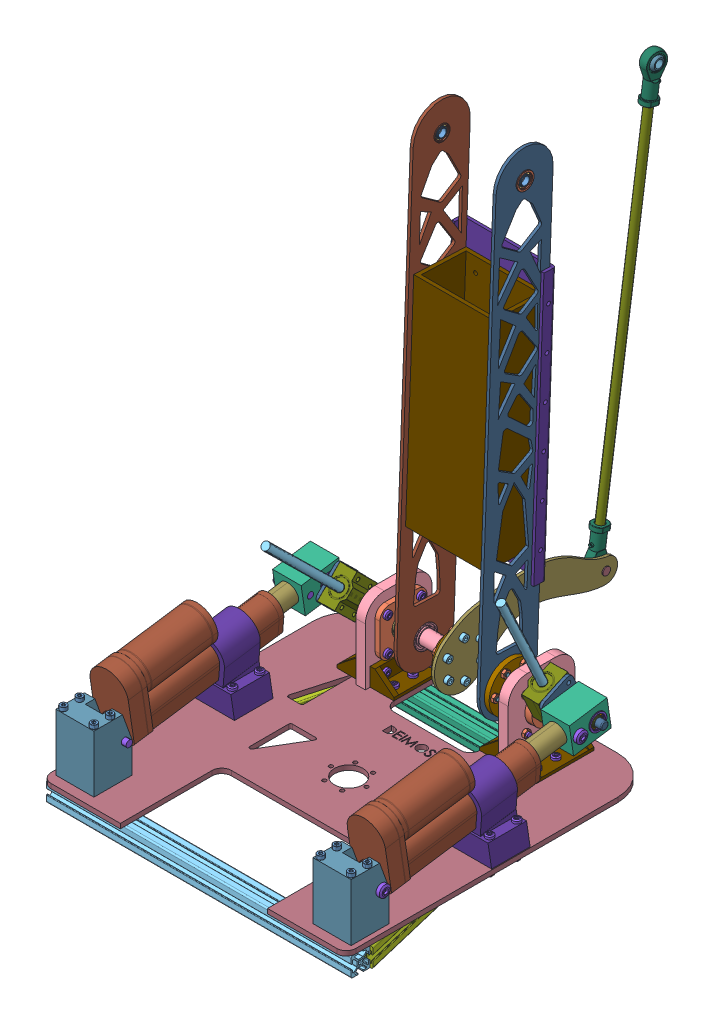
SolidWorks assembly Base + Link1 Final assembly, configuration Default. Lengths in mm. (continued)
Mates (geometry in assembly coordinates): (continued)
- Concentric128: concentric anti-aligned: cylinder of l bracket_arm base flang-4 through (213.5714 103.6403 167.5796) axis (1 0 0) radius 1.6729; cylinder of hexalobular socket pan head_iso-19 through (193.5714 103.6403 167.5796) axis (-1 0 0) radius 2.35
- Coincident132: coincident anti-aligned: plane of l bracket_arm base flang-4 through (218.5714 111.6403 178.5796) normal (1 0 0); plane of hexalobular socket pan head_iso-19 through (218.5714 101.2903 167.5796) normal (-1 0 0)
- Concentric129: concentric anti-aligned: cylinder of l bracket_arm base flang-4 through (213.5714 103.6403 148.5796) axis (1 0 0) radius 1.6729; cylinder of hexalobular socket pan head_iso-20 through (193.5714 103.6403 148.5796) axis (-1 0 0) radius 2.35
- Coincident133: coincident anti-aligned: plane of l bracket_arm base flang-4 through (218.5714 111.6403 178.5796) normal (1 0 0); plane of hexalobular socket pan head_iso-20 through (218.5714 101.2903 148.5796) normal (-1 0 0)
- Concentric130: concentric anti-aligned: cylinder of l bracket_arm base flang-4 through (213.5714 103.6403 129.5796) axis (1 0 0) radius 1.6729; cylinder of hexalobular socket pan head_iso-21 through (193.5714 103.6403 129.5796) axis (-1 0 0) radius 2.35
- Coincident134: coincident anti-aligned: plane of l bracket_arm base flang-4 through (218.5714 111.6403 178.5796) normal (1 0 0); plane of hexalobular socket pan head_iso-21 through (218.5714 101.2903 129.5796) normal (-1 0 0)
- Concentric131: concentric anti-aligned: cylinder of base bearing assambly-2/base shaft bearing housing-1 through (358.5714 155.1403 131.0796) axis (-1 0 0) radius 2; cylinder of hexalobular socket pan head_iso-23 through (368.5714 155.1403 131.0796) axis (1 0 0) radius 2.35
- Coincident135: coincident anti-aligned: plane of base bearing assambly-2/base shaft bearing housing-1 through (348.5714 149.6403 148.5796) normal (-1 0 0); plane of hexalobular socket pan head_iso-23 through (348.5714 157.4903 131.0796) normal (1 0 0)
- Concentric132: concentric anti-aligned: cylinder of base bearing assambly-2/base shaft bearing housing-1 through (358.5714 155.1403 166.0796) axis (-1 0 0) radius 2; cylinder of hexalobular socket pan head_iso-24 through (368.5714 155.1403 166.0796) axis (1 0 0) radius 2.35
- Coincident136: coincident anti-aligned: plane of base bearing assambly-2/base shaft bearing housing-1 through (348.5714 149.6403 148.5796) normal (-1 0 0); plane of hexalobular socket pan head_iso-24 through (348.5714 157.4903 166.0796) normal (1 0 0)
- Concentric133: concentric anti-aligned: cylinder of base bearing assambly-2/base shaft bearing housing-1 through (358.5714 120.1403 131.0796) axis (-1 0 0) radius 2; cylinder of hexalobular socket pan head_iso-25 through (368.5714 120.1403 131.0796) axis (1 0 0) radius 2.35
- Coincident137: coincident anti-aligned: plane of base bearing assambly-2/base shaft bearing housing-1 through (348.5714 149.6403 148.5796) normal (-1 0 0); plane of hexalobular socket pan head_iso-25 through (348.5714 122.4903 131.0796) normal (1 0 0)
- Concentric134: concentric anti-aligned: cylinder of base bearing assambly-2/base shaft bearing housing-1 through (358.5714 120.1403 166.0796) axis (-1 0 0) radius 2; cylinder of hexalobular socket pan head_iso-26 through (368.5714 120.1403 166.0796) axis (1 0 0) radius 2.35
- Coincident138: coincident anti-aligned: plane of base bearing assambly-2/base shaft bearing housing-1 through (348.5714 149.6403 148.5796) normal (-1 0 0); plane of hexalobular socket pan head_iso-26 through (348.5714 122.4903 166.0796) normal (1 0 0)
- Concentric1351: concentric anti-aligned: cylinder of base bearing assambly-1/base shaft bearing housing-1 through (208.5714 120.1403 131.0796) axis (1 0 0) radius 2; cylinder of hexalobular socket pan head_iso-27 through (198.5714 120.1403 131.0796) axis (-1 0 0) radius 2.35
- Coincident1391: coincident anti-aligned: plane of base bearing assambly-1/base shaft bearing housing-1 through (218.5714 149.6403 148.5796) normal (1 0 0); plane of hexalobular socket pan head_iso-27 through (218.5714 117.7903 131.0796) normal (-1 0 0)
- Concentric136: concentric anti-aligned: cylinder of base bearing assambly-1/base shaft bearing housing-1 through (208.5714 155.1403 131.0796) axis (1 0 0) radius 2; cylinder of hexalobular socket pan head_iso-28 through (198.5714 155.1403 131.0796) axis (-1 0 0) radius 2.35
- Coincident140: coincident anti-aligned: plane of base bearing assambly-1/base shaft bearing housing-1 through (218.5714 149.6403 148.5796) normal (1 0 0); plane of hexalobular socket pan head_iso-28 through (218.5714 152.7903 131.0796) normal (-1 0 0)
- Concentric137: concentric anti-aligned: cylinder of base bearing assambly-1/base shaft bearing housing-1 through (208.5714 155.1403 166.0796) axis (1 0 0) radius 2; cylinder of hexalobular socket pan head_iso-29 through (198.5714 155.1403 166.0796) axis (-1 0 0) radius 2.35
- Coincident141: coincident anti-aligned: plane of base bearing assambly-1/base shaft bearing housing-1 through (218.5714 149.6403 148.5796) normal (1 0 0); plane of hexalobular socket pan head_iso-29 through (218.5714 152.7903 166.0796) normal (-1 0 0)
- Concentric138: concentric anti-aligned: cylinder of base bearing assambly-1/base shaft bearing housing-1 through (208.5714 120.1403 166.0796) axis (1 0 0) radius 2; cylinder of hexalobular socket pan head_iso-30 through (198.5714 120.1403 166.0796) axis (-1 0 0) radius 2.35
- Coincident142: coincident anti-aligned: plane of base bearing assambly-1/base shaft bearing housing-1 through (218.5714 149.6403 148.5796) normal (1 0 0); plane of hexalobular socket pan head_iso-30 through (218.5714 117.7903 166.0796) normal (-1 0 0)
- Concentric139: concentric anti-aligned: cylinder of linear_acutator_holder-1 through (437.6971 82.0703 277.3153) axis (0 1 0) radius 2; cylinder of hexalobular socket pan head_iso-32 through (437.6971 83.0703 277.3153) axis (0 -1 0) radius 2.35
- Coincident143: coincident anti-aligned: plane of linear_acutator_holder-1 through (394.6971 118.0703 243.4855) normal (0 1 0); plane of hexalobular socket pan head_iso-32 through (440.0471 118.0703 277.3153) normal (0 -1 0)
- Concentric140: concentric anti-aligned: cylinder of linear_acutator_holder-1 through (437.6971 82.0703 248.7068) axis (0 1 0) radius 2; cylinder of hexalobular socket pan head_iso-33 through (437.6971 83.0703 248.7068) axis (0 -1 0) radius 2.35
- Coincident144: coincident anti-aligned: plane of linear_acutator_holder-1 through (394.6971 118.0703 243.4855) normal (0 1 0); plane of hexalobular socket pan head_iso-33 through (440.0471 118.0703 248.7068) normal (0 -1 0)
- Concentric141: concentric anti-aligned: cylinder of linear_acutator_holder-1 through (399.6971 82.0703 277.3153) axis (0 1 0) radius 2; cylinder of hexalobular socket pan head_iso-34 through (399.6971 83.0703 277.3153) axis (0 -1 0) radius 2.35
- Coincident145: coincident anti-aligned: plane of linear_acutator_holder-1 through (394.6971 118.0703 243.4855) normal (0 1 0); plane of hexalobular socket pan head_iso-34 through (402.0471 118.0703 277.3153) normal (0 -1 0)
- Concentric142: concentric anti-aligned: cylinder of linear_acutator_holder-1 through (399.6971 82.0703 248.7068) axis (0 1 0) radius 2; cylinder of hexalobular socket pan head_iso-35 through (399.6971 83.0703 248.7068) axis (0 -1 0) radius 2.35
- Coincident146: coincident anti-aligned: plane of linear_acutator_holder-1 through (394.6971 118.0703 243.4855) normal (0 1 0); plane of hexalobular socket pan head_iso-35 through (402.0471 118.0703 248.7068) normal (0 -1 0)
- Concentric143: concentric anti-aligned: cylinder of linear_acutator_holder-2 through (129.6971 82.0703 248.7068) axis (0 1 0) radius 2; cylinder of hexalobular socket pan head_iso-36 through (129.6971 83.0703 248.7068) axis (0 -1 0) radius 2.35
- Coincident147: coincident anti-aligned: plane of linear_acutator_holder-2 through (124.6971 118.0703 243.4855) normal (0 1 0); plane of hexalobular socket pan head_iso-36 through (132.0471 118.0703 248.7068) normal (0 -1 0)
- Concentric144: concentric anti-aligned: cylinder of linear_acutator_holder-2 through (129.6971 82.0703 277.3153) axis (0 1 0) radius 2; cylinder of hexalobular socket pan head_iso-37 through (129.6971 83.0703 277.3153) axis (0 -1 0) radius 2.35
- Coincident148: coincident anti-aligned: plane of linear_acutator_holder-2 through (124.6971 118.0703 243.4855) normal (0 1 0); plane of hexalobular socket pan head_iso-37 through (132.0471 118.0703 277.3153) normal (0 -1 0)
- Concentric145: concentric anti-aligned: cylinder of linear_acutator_holder-2 through (167.6971 82.0703 248.7068) axis (0 1 0) radius 2; cylinder of hexalobular socket pan head_iso-38 through (167.6971 83.0703 248.7068) axis (0 -1 0) radius 2.35
- Coincident149: coincident anti-aligned: plane of linear_acutator_holder-2 through (124.6971 118.0703 243.4855) normal (0 1 0); plane of hexalobular socket pan head_iso-38 through (170.0471 118.0703 248.7068) normal (0 -1 0)
- Concentric146: concentric anti-aligned: cylinder of linear_acutator_holder-2 through (167.6971 82.0703 277.3153) axis (0 1 0) radius 2; cylinder of hexalobular socket pan head_iso-39 through (167.6971 83.0703 277.3153) axis (0 -1 0) radius 2.35
- Coincident150: coincident anti-aligned: plane of linear_acutator_holder-2 through (124.6971 118.0703 243.4855) normal (0 1 0); plane of hexalobular socket pan head_iso-39 through (170.0471 118.0703 277.3153) normal (0 -1 0)
- Concentric147: concentric anti-aligned: cylinder of Connector to Linear bearing-1/V8_connectorURC 2024_V4-1 through (234.5714 157.4228 190.9544) axis (-1 0 0) radius 3; cylinder of hexalobular socket pan head_iso-41 through (163.5714 157.4228 190.9544) axis (1 0 0) radius 3.4
- Coincident151: coincident anti-aligned: plane of Connector to Linear bearing-1/V8_connectorURC 2024_V4-1 through (133.5714 176.977 161.4071) normal (-1 0 0); plane of hexalobular socket pan head_iso-41 through (133.5714 160.8228 190.9544) normal (1 0 0)
- Concentric148: concentric aligned: cylinder of Connector to Linear bearing-2/V8_connectorURC 2024_V4-1 through (504.5714 159.1459 179.3562) axis (-1 0 0) radius 3; cylinder of hexalobular socket pan head_iso-42 through (403.5714 159.1459 179.3562) axis (-1 0 0) radius 3.4
- Coincident152: coincident anti-aligned: plane of Connector to Linear bearing-2/V8_connectorURC 2024_V4-1 through (433.5714 178.7 149.8089) normal (1 0 0); plane of hexalobular socket pan head_iso-42 through (433.5714 155.7459 179.3562) normal (-1 0 0)
- Concentric149: concentric aligned: cylinder of hexalobular socket pan head_iso-17 through (373.5714 103.6403 148.5796) axis (1 0 0) radius 2.35; cylinder of hex nut style 1 gradeab_iso-24 through (346.7339 103.6403 148.5796) axis (1 0 0) radius 2
- Coincident153: coincident anti-aligned: plane of l bracket_arm base flang-1 through (368.5714 111.6403 178.5796) normal (1 0 0); plane of hex nut style 1 gradeab_iso-24 through (368.5714 97.2267 145.7749) normal (-1 0 0)
- Concentric150: concentric aligned: cylinder of hexalobular socket pan head_iso-18 through (373.5714 103.6403 167.5796) axis (1 0 0) radius 2.35; cylinder of hex nut style 1 gradeab_iso-25 through (346.7339 103.6403 167.5796) axis (1 0 0) radius 2
- Coincident154: coincident anti-aligned: plane of l bracket_arm base flang-1 through (368.5714 111.6403 178.5796) normal (1 0 0); plane of hex nut style 1 gradeab_iso-25 through (368.5714 103.6403 174.5796) normal (-1 0 0)
- Concentric151: concentric aligned: cylinder of hexalobular socket pan head_iso-16 through (373.5714 103.6403 129.5796) axis (1 0 0) radius 2.35; cylinder of hex nut style 1 gradeab_iso-26 through (346.7339 103.6403 129.5796) axis (1 0 0) radius 2
- Coincident155: coincident anti-aligned: plane of l bracket_arm base flang-1 through (368.5714 111.6403 178.5796) normal (1 0 0); plane of hex nut style 1 gradeab_iso-26 through (368.5714 103.6403 136.5796) normal (-1 0 0)
- Concentric152: concentric anti-aligned: cylinder of base bearing assambly-2/base shaft bearing housing-1 through (358.5714 120.1403 131.0796) axis (-1 0 0) radius 2; cylinder of hex nut style 1 gradeab_iso-27 through (341.7339 120.1403 131.0796) axis (1 0 0) radius 2
- Concentric153: concentric aligned: cylinder of hexalobular socket pan head_iso-23 through (368.5714 155.1403 131.0796) axis (1 0 0) radius 2.35; cylinder of hex nut style 1 gradeab_iso-28 through (341.7339 155.1403 131.0796) axis (1 0 0) radius 2
- Coincident157: coincident anti-aligned: plane of V8_bearing holder holderURC 2024_V4-2 through (363.5714 172.6403 183.5796) normal (1 0 0); plane of hex nut style 1 gradeab_iso-28 through (363.5714 150.101 135.9382) normal (-1 0 0)
- Concentric154: concentric aligned: cylinder of hexalobular socket pan head_iso-24 through (368.5714 155.1403 166.0796) axis (1 0 0) radius 2.35; cylinder of hex nut style 1 gradeab_iso-29 through (341.7339 155.1403 166.0796) axis (1 0 0) radius 2
- Coincident158: coincident anti-aligned: plane of V8_bearing holder holderURC 2024_V4-2 through (363.5714 172.6403 183.5796) normal (1 0 0); plane of hex nut style 1 gradeab_iso-29 through (363.5714 155.1403 173.0796) normal (-1 0 0)
- Concentric155: concentric aligned: cylinder of hexalobular socket pan head_iso-4 through (378.5714 83.6403 128.5796) axis (0 -1 0) radius 2.35; cylinder of hex nut style 1 gradeab_iso-30 through (378.5714 109.4778 128.5796) axis (0 -1 0) radius 2
- Coincident159: coincident anti-aligned: plane of V8_base plate for LAURC 2024_V4-1 through (283.5714 87.6403 412.2334) normal (0 -1 0); plane of hex nut style 1 gradeab_iso-30 through (371.5714 87.6403 128.5796) normal (0 1 0)
- Concentric156: concentric aligned: cylinder of hexalobular socket pan head_iso-7 through (338.5714 83.6403 128.5796) axis (0 -1 0) radius 2.35; cylinder of hex nut style 1 gradeab_iso-31 through (338.5714 109.4778 128.5796) axis (0 -1 0) radius 2
- Coincident160: coincident anti-aligned: plane of V8_base plate for LAURC 2024_V4-1 through (283.5714 87.6403 412.2334) normal (0 -1 0); plane of hex nut style 1 gradeab_iso-31 through (331.5714 87.6403 128.5796) normal (0 1 0)
- Concentric157: concentric aligned: cylinder of hexalobular socket pan head_iso-5 through (338.5714 83.6403 168.5796) axis (0 -1 0) radius 2.35; cylinder of hex nut style 1 gradeab_iso-32 through (338.5714 109.4778 168.5796) axis (0 -1 0) radius 2
- Coincident161: coincident anti-aligned: plane of V8_base plate for LAURC 2024_V4-1 through (283.5714 87.6403 412.2334) normal (0 -1 0); plane of hex nut style 1 gradeab_iso-32 through (331.5714 87.6403 168.5796) normal (0 1 0)
- Coincident163: coincident anti-aligned: plane of V8_bearing holder holderURC 2024_V4-2 through (363.5714 172.6403 183.5796) normal (1 0 0); plane of hex nut style 1 gradeab_iso-27 through (363.5714 120.1403 138.0796) normal (-1 0 0)
- Concentric158: concentric aligned: cylinder of hexalobular socket pan head_iso-26 through (368.5714 120.1403 166.0796) axis (1 0 0) radius 2.35; cylinder of hex nut style 1 gradeab_iso-34 through (341.7339 120.1403 166.0796) axis (1 0 0) radius 2
- Coincident164: coincident anti-aligned: plane of V8_bearing holder holderURC 2024_V4-2 through (363.5714 172.6403 183.5796) normal (1 0 0); plane of hex nut style 1 gradeab_iso-34 through (363.5714 120.1403 173.0796) normal (-1 0 0)
- Concentric159: concentric aligned: cylinder of V8_bearing holder holderURC 2024_V4-1 through (213.5714 155.1403 131.0796) axis (-1 0 0) radius 2; cylinder of hex nut style 1 gradeab_iso-35 through (225.409 155.1403 131.0796) axis (-1 0 0) radius 2
- Coincident165: coincident anti-aligned: plane of V8_bearing holder holderURC 2024_V4-1 through (203.5714 172.6403 113.5796) normal (-1 0 0); plane of hex nut style 1 gradeab_iso-35 through (203.5714 155.1403 124.0796) normal (1 0 0)
- Concentric160: concentric aligned: cylinder of V8_bearing holder holderURC 2024_V4-1 through (213.5714 120.1403 131.0796) axis (-1 0 0) radius 2; cylinder of hex nut style 1 gradeab_iso-36 through (225.409 120.1403 131.0796) axis (-1 0 0) radius 2
- Coincident166: coincident anti-aligned: plane of V8_bearing holder holderURC 2024_V4-1 through (203.5714 172.6403 113.5796) normal (-1 0 0); plane of hex nut style 1 gradeab_iso-36 through (203.5714 120.1403 124.0796) normal (1 0 0)
- Concentric161: concentric aligned: cylinder of V8_bearing holder holderURC 2024_V4-1 through (213.5714 155.1403 166.0796) axis (-1 0 0) radius 2; cylinder of hex nut style 1 gradeab_iso-37 through (225.409 155.1403 166.0796) axis (-1 0 0) radius 2
- Coincident167: coincident anti-aligned: plane of V8_bearing holder holderURC 2024_V4-1 through (203.5714 172.6403 113.5796) normal (-1 0 0); plane of hex nut style 1 gradeab_iso-37 through (203.5714 155.1403 159.0796) normal (1 0 0)
- Concentric162: concentric aligned: cylinder of V8_bearing holder holderURC 2024_V4-1 through (213.5714 120.1403 166.0796) axis (-1 0 0) radius 2; cylinder of hex nut style 1 gradeab_iso-38 through (225.409 120.1403 166.0796) axis (-1 0 0) radius 2
- Coincident168: coincident anti-aligned: plane of V8_bearing holder holderURC 2024_V4-1 through (203.5714 172.6403 113.5796) normal (-1 0 0); plane of hex nut style 1 gradeab_iso-38 through (203.5714 120.1403 159.0796) normal (1 0 0)
- Concentric163: concentric aligned: cylinder of l bracket_arm base flang-3 through (203.5714 103.6403 148.5796) axis (-1 0 0) radius 1.6729; cylinder of hex nut style 1 gradeab_iso-39 through (220.409 103.6403 148.5796) axis (-1 0 0) radius 2
- Coincident169: coincident anti-aligned: plane of l bracket_arm base flang-3 through (198.5714 111.6403 118.5796) normal (-1 0 0); plane of hex nut style 1 gradeab_iso-39 through (198.5714 103.6403 141.5796) normal (1 0 0)
- Concentric164: concentric aligned: cylinder of l bracket_arm base flang-3 through (203.5714 103.6403 167.5796) axis (-1 0 0) radius 1.6729; cylinder of hex nut style 1 gradeab_iso-40 through (220.409 103.6403 167.5796) axis (-1 0 0) radius 2
- Coincident170: coincident anti-aligned: plane of l bracket_arm base flang-3 through (198.5714 111.6403 118.5796) normal (-1 0 0); plane of hex nut style 1 gradeab_iso-40 through (198.5714 103.6403 160.5796) normal (1 0 0)
- Concentric165: concentric aligned: cylinder of l bracket_arm base flang-3 through (203.5714 103.6403 129.5796) axis (-1 0 0) radius 1.6729; cylinder of hex nut style 1 gradeab_iso-41 through (220.409 103.6403 129.5796) axis (-1 0 0) radius 2
- Coincident171: coincident anti-aligned: plane of l bracket_arm base flang-3 through (198.5714 111.6403 118.5796) normal (-1 0 0); plane of hex nut style 1 gradeab_iso-41 through (198.5714 103.6403 122.5796) normal (1 0 0)
- Concentric166: concentric aligned: cylinder of hexalobular socket pan head_iso-8 through (228.5714 83.6403 128.5796) axis (0 -1 0) radius 2.35; cylinder of hex nut style 1 gradeab_iso-42 through (228.5714 109.4778 128.5796) axis (0 -1 0) radius 2
- Coincident172: coincident anti-aligned: plane of V8_base plate for LAURC 2024_V4-1 through (283.5714 87.6403 412.2334) normal (0 -1 0); plane of hex nut style 1 gradeab_iso-42 through (221.5714 87.6403 128.5796) normal (0 1 0)
- Concentric167: concentric aligned: cylinder of hexalobular socket pan head_iso-11 through (188.5714 83.6403 128.5796) axis (0 -1 0) radius 2.35; cylinder of hex nut style 1 gradeab_iso-43 through (188.5714 109.4778 128.5796) axis (0 -1 0) radius 2
- Coincident173: coincident anti-aligned: plane of V8_base plate for LAURC 2024_V4-1 through (283.5714 87.6403 412.2334) normal (0 -1 0); plane of hex nut style 1 gradeab_iso-43 through (181.5714 87.6403 128.5796) normal (0 1 0)
- Concentric168: concentric aligned: cylinder of hexalobular socket pan head_iso-10 through (228.5714 83.6403 168.5796) axis (0 -1 0) radius 2.35; cylinder of hex nut style 1 gradeab_iso-44 through (228.5714 109.4778 168.5796) axis (0 -1 0) radius 2
- Coincident174: coincident anti-aligned: plane of V8_base plate for LAURC 2024_V4-1 through (283.5714 87.6403 412.2334) normal (0 -1 0); plane of hex nut style 1 gradeab_iso-44 through (221.5714 87.6403 168.5796) normal (0 1 0)
- Concentric169: concentric aligned: cylinder of hexalobular socket pan head_iso-37 through (129.6971 83.0703 277.3153) axis (0 -1 0) radius 2.35; cylinder of hex nut style 1 gradeab_iso-45 through (129.6971 109.4778 277.3153) axis (0 -1 0) radius 2
- Coincident175: coincident anti-aligned: plane of V8_base plate for LAURC 2024_V4-1 through (283.5714 87.6403 412.2334) normal (0 -1 0); plane of hex nut style 1 gradeab_iso-45 through (122.6971 87.6403 277.3153) normal (0 1 0)
- Concentric170: concentric aligned: cylinder of hexalobular socket pan head_iso-36 through (129.6971 83.0703 248.7068) axis (0 -1 0) radius 2.35; cylinder of hex nut style 1 gradeab_iso-46 through (129.6971 109.4778 248.7068) axis (0 -1 0) radius 2
- Coincident176: coincident anti-aligned: plane of V8_base plate for LAURC 2024_V4-1 through (283.5714 87.6403 412.2334) normal (0 -1 0); plane of hex nut style 1 gradeab_iso-46 through (122.6971 87.6403 248.7068) normal (0 1 0)
- Concentric171: concentric anti-aligned: cylinder of linear_acutator_holder-1 through (437.6971 82.0703 277.3153) axis (0 1 0) radius 2; cylinder of hex nut style 1 gradeab_iso-47 through (437.6971 109.4778 277.3153) axis (0 -1 0) radius 2
- Concentric172: concentric anti-aligned: cylinder of V8_base plate for LAURC 2024_V4-1 through (437.4458 87.6403 248.7068) axis (0 1 0) radius 2; cylinder of hex nut style 1 gradeab_iso-48 through (437.4458 109.4778 248.7068) axis (0 -1 0) radius 2
- Coincident178: coincident anti-aligned: plane of V8_base plate for LAURC 2024_V4-1 through (283.5714 87.6403 412.2334) normal (0 -1 0); plane of hex nut style 1 gradeab_iso-48 through (436.8655 87.6403 255.6827) normal (0 1 0)
- Coincident179: coincident anti-aligned: plane of V8_base plate for LAURC 2024_V4-1 through (283.5714 87.6403 412.2334) normal (0 -1 0); plane of hex nut style 1 gradeab_iso-47 through (439.9519 87.6403 283.9422) normal (0 1 0)
- Concentric173: concentric anti-aligned: cylinder of LA_back holder-1 through (196.5714 127.6403 391.4309) axis (-1 0 0) radius 3; cylinder of hexalobular socket pan head_iso-44 through (173.5714 127.6403 391.4309) axis (1 0 0) radius 3.4
- Coincident180: coincident anti-aligned: plane of LA_back holder-1 through (128.5714 92.6403 403.5796) normal (-1 0 0); plane of hexalobular socket pan head_iso-44 through (128.5714 131.0403 391.4309) normal (1 0 0)
- Concentric174: concentric aligned: cylinder of LA_back holder-2 through (466.5714 127.6403 391.4309) axis (-1 0 0) radius 3; cylinder of hexalobular socket pan head_iso-45 through (393.5714 127.6403 391.4309) axis (-1 0 0) radius 3.4
- Coincident181: coincident anti-aligned: plane of LA_back holder-2 through (438.5714 92.6403 403.5796) normal (1 0 0); plane of hexalobular socket pan head_iso-45 through (438.5714 124.2403 391.4309) normal (-1 0 0)
- Concentric1352: concentric aligned: cylinder of V8_shaftURC 2024_V4 real part-1 through (333.5714 137.6403 148.5796) axis (-1 0 0) radius 7.5; cylinder of Base Shaft connector to link 1-1 through (343.5714 137.6403 148.5796) axis (-1 0 0) radius 7.5
- Coincident1393: coincident aligned: plane of V8_base plate for LAURC 2024_V4-1 through (328.5714 97.6403 188.5796) normal (-1 0 0); plane of Base Shaft connector to link 1-1 through (328.5714 137.6403 148.5796) normal (-1 0 0)
- Concentric1353: concentric anti-aligned: circle of V8_shaftURC 2024_V4-1; circle of lock_nut_for coupler-3
- Coincident1394: coincident anti-aligned: plane of linnear rod coupler-1 through (170.8714 137.6403 148.5796) normal (-1 0 0); plane of lock_nut_for coupler-3 through (170.8714 137.6403 148.5796) normal (1 0 0)
- Concentric1354: concentric anti-aligned: cylinder of V8_shaftURC 2024_V4-1 through (273.0714 137.6403 148.5796) axis (1 0 0) radius 7.5; circle of Base Shaft connector to link 1-2
- Coincident1395: coincident anti-aligned: plane of V8_shaftURC 2024_V4-1 through (273.0714 144.9751 150.1451) normal (1 0 0); plane of Base Shaft connector to link 1-2 through (273.0714 137.6403 148.5796) normal (-1 0 0)
- Concentric1355: concentric anti-aligned: cylinder of V8_shaftURC 2024_V4 real part-1 through (333.5714 137.6403 148.5796) axis (-1 0 0) radius 7.5; cylinder of Link 1 assmebly-1/V8_link 1_real_transmisionURC 2024-1 through (325.5714 137.6403 148.5796) axis (1 0 0) radius 8
- Coincident1396: coincident anti-aligned: plane of Base Shaft connector to link 1-1 through (328.5714 137.6403 148.5796) normal (-1 0 0); plane of Link 1 assmebly-1/V8_link 1_real_transmisionURC 2024-1 through (328.5714 137.6403 148.5796) normal (1 0 0)
- Concentric1356: concentric anti-aligned: cylinder of Base Shaft connector to link 1-1 through (333.5714 154.5674 137.9272) axis (-1 0 0) radius 2; cylinder of Link 1 assmebly-1/V8_link 1_real_transmisionURC 2024-1 through (325.5714 154.5674 137.9272) axis (1 0 0) radius 2
- Concentric1357: concentric anti-aligned: cylinder of Link 1 assmebly-1/V8_link 1_fack_transmisionURC 2024-1 through (241.5714 137.6403 148.5796) axis (-1 0 0) radius 12; cylinder of radial ball bearing_68_iso-1 through (219.4339 137.6403 148.5796) axis (1 0 0) radius 12
- Distance22: distance = 1 mm aligned: plane of radial ball bearing_68_iso-1 through (242.5714 149.3403 148.5796) normal (1 0 0); plane of Link 1 assmebly-1/V8_link 1_fack_transmisionURC 2024-1 through (241.5714 137.6403 148.5796) normal (1 0 0)
- Concentric1358: concentric anti-aligned: cylinder of Base Shaft connector to link 1-2 through (273.0714 148.1762 131.5798) axis (1 0 0) radius 2; cylinder of Link 1 assmebly-1/V8_link_2_power_rod_1_v4URC 2024-1 through (281.0714 148.1762 131.5798) axis (-1 0 0) radius 2
- Concentric1359: concentric anti-aligned: cylinder of Link 1 assmebly-1/V8_link 1_real_transmisionURC 2024-1 through (325.5714 154.5674 137.9272) axis (1 0 0) radius 2; cylinder of socket head cap screw_iso-2 through (289.8214 154.5674 137.9272) axis (-1 0 0) radius 3.5
- Coincident1397: coincident anti-aligned: plane of Link 1 assmebly-1/V8_link 1_real_transmisionURC 2024-1 through (325.5714 137.6403 148.5796) normal (-1 0 0); plane of socket head cap screw_iso-2 through (325.5714 158.0674 137.9272) normal (1 0 0)
- Concentric1360: concentric anti-aligned: cylinder of Link 1 assmebly-1/V8_link 1_real_transmisionURC 2024-1 through (325.5714 155.329 157.9127) axis (1 0 0) radius 2; cylinder of socket head cap screw_iso-3 through (289.8214 155.329 157.9127) axis (-1 0 0) radius 3.5
- Coincident1398: coincident anti-aligned: plane of Link 1 assmebly-1/V8_link 1_real_transmisionURC 2024-1 through (325.5714 137.6403 148.5796) normal (-1 0 0); plane of socket head cap screw_iso-3 through (325.5714 158.829 157.9127) normal (1 0 0)
- Concentric1361: concentric anti-aligned: cylinder of Link 1 assmebly-1/V8_link 1_real_transmisionURC 2024-1 through (325.5714 138.4019 168.5651) axis (1 0 0) radius 2; cylinder of socket head cap screw_iso-4 through (289.8214 138.4019 168.5651) axis (-1 0 0) radius 3.5
- Coincident1399: coincident anti-aligned: plane of Link 1 assmebly-1/V8_link 1_real_transmisionURC 2024-1 through (325.5714 137.6403 148.5796) normal (-1 0 0); plane of socket head cap screw_iso-4 through (325.5714 141.9019 168.5651) normal (1 0 0)
- Concentric1362: concentric anti-aligned: cylinder of Link 1 assmebly-1/V8_link 1_real_transmisionURC 2024-1 through (325.5714 120.7132 159.232) axis (1 0 0) radius 2; cylinder of socket head cap screw_iso-5 through (289.8214 120.7132 159.232) axis (-1 0 0) radius 3.5
- Coincident1400: coincident anti-aligned: plane of Link 1 assmebly-1/V8_link 1_real_transmisionURC 2024-1 through (325.5714 137.6403 148.5796) normal (-1 0 0); plane of socket head cap screw_iso-5 through (325.5714 124.2132 159.232) normal (1 0 0)
- Concentric1363: concentric anti-aligned: cylinder of Link 1 assmebly-1/V8_link 1_real_transmisionURC 2024-1 through (325.5714 119.9515 139.2465) axis (1 0 0) radius 2; cylinder of socket head cap screw_iso-6 through (289.8214 119.9515 139.2465) axis (-1 0 0) radius 3.5
- Coincident1401: coincident anti-aligned: plane of Link 1 assmebly-1/V8_link 1_real_transmisionURC 2024-1 through (325.5714 137.6403 148.5796) normal (-1 0 0); plane of socket head cap screw_iso-6 through (325.5714 123.4515 139.2465) normal (1 0 0)
- Concentric1364: concentric anti-aligned: cylinder of Link 1 assmebly-1/V8_link 1_real_transmisionURC 2024-1 through (325.5714 136.8786 128.5941) axis (1 0 0) radius 2; cylinder of socket head cap screw_iso-7 through (289.8214 136.8786 128.5941) axis (-1 0 0) radius 3.5
- Coincident1402: coincident anti-aligned: plane of Link 1 assmebly-1/V8_link 1_real_transmisionURC 2024-1 through (325.5714 137.6403 148.5796) normal (-1 0 0); plane of socket head cap screw_iso-7 through (325.5714 140.3786 128.5941) normal (1 0 0)
- Concentric1365: concentric anti-aligned: cylinder of Link 1 assmebly-1/V8_link_2_power_rod_1_v4URC 2024-1 through (281.0714 157.6305 149.2041) axis (-1 0 0) radius 2; cylinder of socket head cap screw_iso-8 through (316.8214 157.6305 149.2041) axis (1 0 0) radius 3.5
- Coincident1403: coincident anti-aligned: plane of Link 1 assmebly-1/V8_link_2_power_rod_1_v4URC 2024-1 through (281.0714 137.6403 148.5796) normal (1 0 0); plane of socket head cap screw_iso-8 through (281.0714 156.294 152.4389) normal (-1 0 0)
- Concentric1366: concentric anti-aligned: cylinder of Link 1 assmebly-1/V8_link_2_power_rod_1_v4URC 2024-1 through (281.0714 148.1762 131.5798) axis (-1 0 0) radius 2; cylinder of socket head cap screw_iso-9 through (316.8214 148.1762 131.5798) axis (1 0 0) radius 3.5
- Coincident1404: coincident anti-aligned: plane of Link 1 assmebly-1/V8_link_2_power_rod_1_v4URC 2024-1 through (281.0714 137.6403 148.5796) normal (1 0 0); plane of socket head cap screw_iso-9 through (281.0714 146.8397 134.8146) normal (-1 0 0)
- Concentric1367: concentric anti-aligned: cylinder of Link 1 assmebly-1/V8_link_2_power_rod_1_v4URC 2024-1 through (281.0714 128.186 130.9553) axis (-1 0 0) radius 2; cylinder of socket head cap screw_iso-10 through (316.8214 128.186 130.9553) axis (1 0 0) radius 3.5
- Coincident1405: coincident anti-aligned: plane of Link 1 assmebly-1/V8_link_2_power_rod_1_v4URC 2024-1 through (281.0714 137.6403 148.5796) normal (1 0 0); plane of socket head cap screw_iso-10 through (281.0714 126.8495 134.1901) normal (-1 0 0)
- Concentric1368: concentric anti-aligned: cylinder of Link 1 assmebly-1/V8_link_2_power_rod_1_v4URC 2024-1 through (281.0714 117.65 147.9551) axis (-1 0 0) radius 2; cylinder of socket head cap screw_iso-11 through (316.8214 117.65 147.9551) axis (1 0 0) radius 3.5
- Coincident1406: coincident anti-aligned: plane of Link 1 assmebly-1/V8_link_2_power_rod_1_v4URC 2024-1 through (281.0714 137.6403 148.5796) normal (1 0 0); plane of socket head cap screw_iso-11 through (281.0714 116.3136 151.1899) normal (-1 0 0)
- Concentric1369: concentric anti-aligned: cylinder of Link 1 assmebly-1/V8_link_2_power_rod_1_v4URC 2024-1 through (281.0714 127.1043 165.5794) axis (-1 0 0) radius 2; cylinder of socket head cap screw_iso-12 through (316.8214 127.1043 165.5794) axis (1 0 0) radius 3.5
- Coincident1407: coincident anti-aligned: plane of Link 1 assmebly-1/V8_link_2_power_rod_1_v4URC 2024-1 through (281.0714 137.6403 148.5796) normal (1 0 0); plane of socket head cap screw_iso-12 through (281.0714 125.7679 168.8142) normal (-1 0 0)
- Concentric1370: concentric anti-aligned: cylinder of Link 1 assmebly-1/V8_link_2_power_rod_1_v4URC 2024-1 through (281.0714 147.0946 166.2039) axis (-1 0 0) radius 2; cylinder of socket head cap screw_iso-13 through (316.8214 147.0946 166.2039) axis (1 0 0) radius 3.5
- Coincident1408: coincident anti-aligned: plane of Link 1 assmebly-1/V8_link_2_power_rod_1_v4URC 2024-1 through (281.0714 137.6403 148.5796) normal (1 0 0); plane of socket head cap screw_iso-13 through (281.0714 145.7581 169.4387) normal (-1 0 0)
- Concentric1371: concentric anti-aligned: cylinder of Base Shaft connector to link 1-2 through (273.0714 148.1762 131.5798) axis (1 0 0) radius 2; cylinder of hex nut style 1 gradeab_iso-50 through (294.909 148.1762 131.5798) axis (-1 0 0) radius 2
- Coincident1409: coincident anti-aligned: plane of Base Shaft connector to link 1-2 through (273.0714 137.6403 148.5796) normal (-1 0 0); plane of hex nut style 1 gradeab_iso-50 through (273.0714 148.1762 124.5798) normal (1 0 0)
- Concentric1372: concentric anti-aligned: cylinder of Base Shaft connector to link 1-2 through (273.0714 157.6305 149.2041) axis (1 0 0) radius 2; cylinder of hex nut style 1 gradeab_iso-51 through (294.909 157.6305 149.2041) axis (-1 0 0) radius 2
- Coincident1410: coincident anti-aligned: plane of Base Shaft connector to link 1-2 through (273.0714 137.6403 148.5796) normal (-1 0 0); plane of hex nut style 1 gradeab_iso-51 through (273.0714 157.6305 142.2041) normal (1 0 0)
- Concentric1373: concentric anti-aligned: cylinder of Base Shaft connector to link 1-2 through (273.0714 147.0946 166.2039) axis (1 0 0) radius 2; cylinder of hex nut style 1 gradeab_iso-52 through (294.909 147.0946 166.2039) axis (-1 0 0) radius 2
- Coincident1411: coincident anti-aligned: plane of Base Shaft connector to link 1-2 through (273.0714 137.6403 148.5796) normal (-1 0 0); plane of hex nut style 1 gradeab_iso-52 through (273.0714 147.0946 159.2039) normal (1 0 0)
- Concentric1374: concentric anti-aligned: cylinder of Base Shaft connector to link 1-2 through (273.0714 127.1043 165.5794) axis (1 0 0) radius 2; cylinder of hex nut style 1 gradeab_iso-53 through (294.909 127.1043 165.5794) axis (-1 0 0) radius 2
- Coincident1412: coincident anti-aligned: plane of Base Shaft connector to link 1-2 through (273.0714 137.6403 148.5796) normal (-1 0 0); plane of hex nut style 1 gradeab_iso-53 through (273.0714 127.1043 158.5794) normal (1 0 0)
- Concentric1375: concentric anti-aligned: cylinder of Base Shaft connector to link 1-2 through (273.0714 117.65 147.9551) axis (1 0 0) radius 2; cylinder of hex nut style 1 gradeab_iso-54 through (294.909 117.65 147.9551) axis (-1 0 0) radius 2
- Coincident1413: coincident anti-aligned: plane of Base Shaft connector to link 1-2 through (273.0714 137.6403 148.5796) normal (-1 0 0); plane of hex nut style 1 gradeab_iso-54 through (273.0714 117.65 140.9551) normal (1 0 0)
- Concentric1376: concentric anti-aligned: cylinder of Base Shaft connector to link 1-2 through (273.0714 128.186 130.9553) axis (1 0 0) radius 2; cylinder of hex nut style 1 gradeab_iso-55 through (294.909 128.186 130.9553) axis (-1 0 0) radius 2
- Coincident1414: coincident anti-aligned: plane of Base Shaft connector to link 1-2 through (273.0714 137.6403 148.5796) normal (-1 0 0); plane of hex nut style 1 gradeab_iso-55 through (273.0714 128.186 123.9553) normal (1 0 0)
- Concentric1377: concentric anti-aligned: cylinder of Base Shaft connector to link 1-1 through (333.5714 154.5674 137.9272) axis (-1 0 0) radius 2; cylinder of hex nut style 1 gradeab_iso-56 through (311.7339 154.5674 137.9272) axis (1 0 0) radius 2
- Coincident1415: coincident anti-aligned: plane of Base Shaft connector to link 1-1 through (333.5714 137.6403 148.5796) normal (1 0 0); plane of hex nut style 1 gradeab_iso-56 through (333.5714 154.5674 144.9272) normal (-1 0 0)
- Concentric1378: concentric anti-aligned: cylinder of Base Shaft connector to link 1-1 through (333.5714 136.8786 128.5941) axis (-1 0 0) radius 2; cylinder of hex nut style 1 gradeab_iso-57 through (311.7339 136.8786 128.5941) axis (1 0 0) radius 2
- Coincident1416: coincident anti-aligned: plane of Base Shaft connector to link 1-1 through (333.5714 137.6403 148.5796) normal (1 0 0); plane of hex nut style 1 gradeab_iso-57 through (333.5714 136.8786 135.5941) normal (-1 0 0)
- Concentric1379: concentric anti-aligned: cylinder of Base Shaft connector to link 1-1 through (333.5714 155.329 157.9127) axis (-1 0 0) radius 2; cylinder of hex nut style 1 gradeab_iso-58 through (311.7339 155.329 157.9127) axis (1 0 0) radius 2
- Coincident1417: coincident anti-aligned: plane of Base Shaft connector to link 1-1 through (333.5714 137.6403 148.5796) normal (1 0 0); plane of hex nut style 1 gradeab_iso-58 through (333.5714 155.329 164.9127) normal (-1 0 0)
- Concentric1380: concentric anti-aligned: cylinder of Base Shaft connector to link 1-1 through (333.5714 119.9515 139.2465) axis (-1 0 0) radius 2; cylinder of hex nut style 1 gradeab_iso-59 through (311.7339 119.9515 139.2465) axis (1 0 0) radius 2
- Coincident1418: coincident anti-aligned: plane of Base Shaft connector to link 1-1 through (333.5714 137.6403 148.5796) normal (1 0 0); plane of hex nut style 1 gradeab_iso-59 through (333.5714 119.9515 146.2465) normal (-1 0 0)
- Concentric1381: concentric anti-aligned: cylinder of Base Shaft connector to link 1-1 through (333.5714 120.7132 159.232) axis (-1 0 0) radius 2; cylinder of hex nut style 1 gradeab_iso-60 through (311.7339 120.7132 159.232) axis (1 0 0) radius 2
- Coincident1419: coincident anti-aligned: plane of Base Shaft connector to link 1-1 through (333.5714 137.6403 148.5796) normal (1 0 0); plane of hex nut style 1 gradeab_iso-60 through (333.5714 120.7132 166.232) normal (-1 0 0)
- Concentric1382: concentric anti-aligned: cylinder of Base Shaft connector to link 1-1 through (333.5714 138.4019 168.5651) axis (-1 0 0) radius 2; cylinder of hex nut style 1 gradeab_iso-61 through (311.7339 138.4019 168.5651) axis (1 0 0) radius 2
- Coincident1420: coincident anti-aligned: plane of Base Shaft connector to link 1-1 through (333.5714 137.6403 148.5796) normal (1 0 0); plane of hex nut style 1 gradeab_iso-61 through (333.5714 138.4019 175.5651) normal (-1 0 0)
